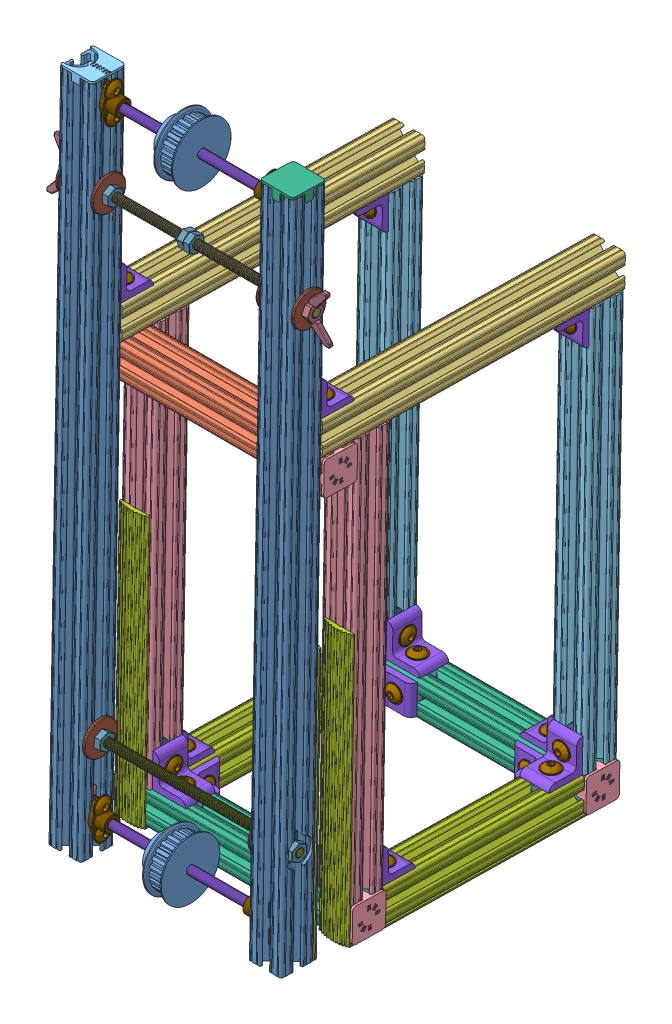
SolidWorks assembly Frame_Assembly_Hardware, configuration Default. Lengths in mm.
Overall size (211.14 529.34 273.97).
180 component instances, 25 part files, 105 mates.
Components (placement in the parent):
- Frame_Extrusions_Assembly-1: Frame_Extrusions_Assembly [Default] at (-237.7441 -252.6867 -297.1575) size (178.82 515.56 261.7)
  - 20in-1: 20in [Default] at (159.5058 -13.8785 410.58) x (1 0 0) z (0 -0.999848 0.017452) size (25.91 25.4 508)
  - 20in-2: 20in [Default] at (311.9058 -13.8785 410.58) x (-1 0 0) z (0 -0.999848 0.017452) size (25.91 25.4 508)
  - 7in_Drilled-1: 7in_Drilled [Default] at (121.4058 325.3515 379.2549) x (0 0.017452 0.999848) z (-1 0 0) size (25.4 25.4 177.8)
  - 9.0625in-1: 9.0625in [Default] at (159.5058 351.4126 416.9058) x (1 0 0) z (0 0.017452 0.999848) size (25.4 25.4 230.19)
  - 9.0625in-2: 9.0625in [Default] at (311.9058 351.4126 416.9058) x (1 0 0) z (0 0.017452 0.999848) size (25.4 25.4 230.19)
  - 12in_Drilled-2: 12in_Drilled [Default] at (159.5058 7.4289 357.8126) x (-1 0 0) z (0 -0.999848 0.017452) size (25.4 25.4 304.8)
  - 12in_Drilled-3: 12in_Drilled [Default] at (311.9058 7.4289 357.8126) x (-1 0 0) z (0 -0.999848 0.017452) size (25.4 25.4 304.8)
  - 12in-1: 12in [Default] at (159.5058 4.3258 180.0397) x (1 0 0) z (0 -0.999848 0.017452) size (25.4 25.4 304.8)
  - 12in-2: 12in [Default] at (311.9058 4.3258 180.0397) x (1 0 0) z (0 -0.999848 0.017452) size (25.4 25.4 304.8)
  - 7in-1: 7in [Default] at (350.0058 20.1269 357.591) x (0 -0.017452 -0.999848) z (1 0 0) size (25.4 25.4 177.8)
  - 7in-2: 7in [Default] at (350.0058 17.0239 179.8181) x (0 -0.017452 -0.999848) z (1 0 0) size (25.4 25.4 177.8)
  - 6in-1: 6in [Default] at (159.5058 20.3486 370.289) x (1 0 0) z (0 0.017452 0.999848) size (25.4 25.4 152.4)
  - 6in-2: 6in [Default] at (311.9058 20.3486 370.289) x (1 0 0) z (0 0.017452 0.999848) size (25.4 25.4 152.4)
- Corner_Brackets_Assembly-1: Corner_Brackets_Assembly [Default] at (64.4635 -222.9732 -111.8459) x (1 0 0) z (0 0.017452 0.999848) size (22.23 33.74 33.74)
  - 2_Hole_Corner_Bracket-1: 2_Hole_Corner_Bracket [Default] at (9.6983 0.1081 6.9858) size (22.23 25.4 25.4)
  - 1_4-20x.5_Flange-1: 1_4-20x.5_Flange [Default] at (9.6983 4.8706 19.6858) x (0 -1 0) z (-0.5 0 0.866025) size (16.15 13.21 13.21)
  - 1_4-20T_Nut-1: 1_4-20T_Nut [Default] at (9.6983 -5.8736 19.6858) x (0 0 1) z (0 -1 0) size (25.4 11.25 3.2)
  - 1_4-20x.5_Flange-2: 1_4-20x.5_Flange [Default] at (9.6983 12.8081 11.7483) x (0 0 -1) z (1 0 0) size (16.15 13.21 13.21)
  - 1_4-20T_Nut-2: 1_4-20T_Nut [Default] at (9.6983 12.8081 1.0041) x (0 1 0) z (0 0 -1) size (25.4 11.25 3.2)
- Corner_Brackets_Assembly-2: Corner_Brackets_Assembly [Default] at (-87.9365 -222.9732 -111.8459) x (1 0 0) z (0 0.017452 0.999848) size (22.23 33.74 33.74)
  - 2_Hole_Corner_Bracket-1: 2_Hole_Corner_Bracket [Default] at (9.6983 0.1081 6.9858) size (22.23 25.4 25.4)
  - 1_4-20x.5_Flange-1: 1_4-20x.5_Flange [Default] at (9.6983 4.8706 19.6858) x (0 -1 0) z (-0.5 0 0.866025) size (16.15 13.21 13.21)
  - 1_4-20T_Nut-1: 1_4-20T_Nut [Default] at (9.6983 -5.8736 19.6858) x (0 0 1) z (0 -1 0) size (25.4 11.25 3.2)
  - 1_4-20x.5_Flange-2: 1_4-20x.5_Flange [Default] at (9.6983 12.8081 11.7483) x (0 0 -1) z (1 0 0) size (16.15 13.21 13.21)
  - 1_4-20T_Nut-2: 1_4-20T_Nut [Default] at (9.6983 12.8081 1.0041) x (0 1 0) z (0 0 -1) size (25.4 11.25 3.2)
- Corner_Brackets_Assembly-3: Corner_Brackets_Assembly [Default] at (83.8601 -220.0696 54.5004) x (-1 0 0) z (0 -0.017452 -0.999848) size (22.23 33.74 33.74)
  - 2_Hole_Corner_Bracket-1: 2_Hole_Corner_Bracket [Default] at (9.6983 0.1081 6.9858) size (22.23 25.4 25.4)
  - 1_4-20x.5_Flange-1: 1_4-20x.5_Flange [Default] at (9.6983 4.8706 19.6858) x (0 -1 0) z (-0.5 0 0.866025) size (16.15 13.21 13.21)
  - 1_4-20T_Nut-1: 1_4-20T_Nut [Default] at (9.6983 -5.8736 19.6858) x (0 0 1) z (0 -1 0) size (25.4 11.25 3.2)
  - 1_4-20x.5_Flange-2: 1_4-20x.5_Flange [Default] at (9.6983 12.8081 11.7483) x (0 0 -1) z (1 0 0) size (16.15 13.21 13.21)
  - 1_4-20T_Nut-2: 1_4-20T_Nut [Default] at (9.6983 12.8081 1.0041) x (0 1 0) z (0 0 -1) size (25.4 11.25 3.2)
- Corner_Brackets_Assembly-4: Corner_Brackets_Assembly [Default] at (-68.5399 -220.0696 54.5004) x (-1 0 0) z (0 -0.017452 -0.999848) size (22.23 33.74 33.74)
  - 2_Hole_Corner_Bracket-1: 2_Hole_Corner_Bracket [Default] at (9.6983 0.1081 6.9858) size (22.23 25.4 25.4)
  - 1_4-20x.5_Flange-1: 1_4-20x.5_Flange [Default] at (9.6983 4.8706 19.6858) x (0 -1 0) z (-0.5 0 0.866025) size (16.15 13.21 13.21)
  - 1_4-20T_Nut-1: 1_4-20T_Nut [Default] at (9.6983 -5.8736 19.6858) x (0 0 1) z (0 -1 0) size (25.4 11.25 3.2)
  - 1_4-20x.5_Flange-2: 1_4-20x.5_Flange [Default] at (9.6983 12.8081 11.7483) x (0 0 -1) z (1 0 0) size (16.15 13.21 13.21)
  - 1_4-20T_Nut-2: 1_4-20T_Nut [Default] at (9.6983 12.8081 1.0041) x (0 1 0) z (0 0 -1) size (25.4 11.25 3.2)
- Corner_Brackets_Assembly-7: Corner_Brackets_Assembly [Default] at (-87.9365 88.9933 -110.4126) x (1 0 0) z (0 -0.999848 0.017452) size (22.23 33.74 33.74)
  - 2_Hole_Corner_Bracket-1: 2_Hole_Corner_Bracket [Default] at (9.6983 0.1081 6.9858) size (22.23 25.4 25.4)
  - 1_4-20x.5_Flange-1: 1_4-20x.5_Flange [Default] at (9.6983 4.8706 19.6858) x (0 -1 0) z (-0.5 0 0.866025) size (16.15 13.21 13.21)
  - 1_4-20T_Nut-1: 1_4-20T_Nut [Default] at (9.6983 -5.8736 19.6858) x (0 0 1) z (0 -1 0) size (25.4 11.25 3.2)
  - 1_4-20x.5_Flange-2: 1_4-20x.5_Flange [Default] at (9.6983 12.8081 11.7483) x (0 0 -1) z (1 0 0) size (16.15 13.21 13.21)
  - 1_4-20T_Nut-2: 1_4-20T_Nut [Default] at (9.6983 12.8081 1.0041) x (0 1 0) z (0 0 -1) size (25.4 11.25 3.2)
- Corner_Brackets_Assembly-8: Corner_Brackets_Assembly [Default] at (64.4635 88.9933 -110.4126) x (1 0 0) z (0 -0.999848 0.017452) size (22.23 33.74 33.74)
  - 2_Hole_Corner_Bracket-1: 2_Hole_Corner_Bracket [Default] at (9.6983 0.1081 6.9858) size (22.23 25.4 25.4)
  - 1_4-20x.5_Flange-1: 1_4-20x.5_Flange [Default] at (9.6983 4.8706 19.6858) x (0 -1 0) z (-0.5 0 0.866025) size (16.15 13.21 13.21)
  - 1_4-20T_Nut-1: 1_4-20T_Nut [Default] at (9.6983 -5.8736 19.6858) x (0 0 1) z (0 -1 0) size (25.4 11.25 3.2)
  - 1_4-20x.5_Flange-2: 1_4-20x.5_Flange [Default] at (9.6983 12.8081 11.7483) x (0 0 -1) z (1 0 0) size (16.15 13.21 13.21)
  - 1_4-20T_Nut-2: 1_4-20T_Nut [Default] at (9.6983 12.8081 1.0041) x (0 1 0) z (0 0 -1) size (25.4 11.25 3.2)
- Corner_Brackets_Assembly-9: Corner_Brackets_Assembly [Default] at (-72.5241 -219.8006 69.9105) x (0 -0.017452 -0.999848) z (1 0 0) size (22.23 33.74 33.74)
  - 2_Hole_Corner_Bracket-1: 2_Hole_Corner_Bracket [Default] at (9.6983 0.1081 6.9858) size (22.23 25.4 25.4)
  - 1_4-20x.5_Flange-1: 1_4-20x.5_Flange [Default] at (9.6983 4.8706 19.6858) x (0 -1 0) z (-0.5 0 0.866025) size (16.15 13.21 13.21)
  - 1_4-20T_Nut-1: 1_4-20T_Nut [Default] at (9.6983 -5.8736 19.6858) x (0 0 1) z (0 -1 0) size (25.4 11.25 3.2)
  - 1_4-20x.5_Flange-2: 1_4-20x.5_Flange [Default] at (9.6983 12.8081 11.7483) x (0 0 -1) z (1 0 0) size (16.15 13.21 13.21)
  - 1_4-20T_Nut-2: 1_4-20T_Nut [Default] at (9.6983 12.8081 1.0041) x (0 1 0) z (0 0 -1) size (25.4 11.25 3.2)
- Corner_Brackets_Assembly-10: Corner_Brackets_Assembly [Default] at (-72.5241 -222.9036 -107.8624) x (0 -0.017452 -0.999848) z (1 0 0) size (22.23 33.74 33.74)
  - 2_Hole_Corner_Bracket-1: 2_Hole_Corner_Bracket [Default] at (9.6983 0.1081 6.9858) size (22.23 25.4 25.4)
  - 1_4-20x.5_Flange-1: 1_4-20x.5_Flange [Default] at (9.6983 4.8706 19.6858) x (0 -1 0) z (-0.5 0 0.866025) size (16.15 13.21 13.21)
  - 1_4-20T_Nut-1: 1_4-20T_Nut [Default] at (9.6983 -5.8736 19.6858) x (0 0 1) z (0 -1 0) size (25.4 11.25 3.2)
  - 1_4-20x.5_Flange-2: 1_4-20x.5_Flange [Default] at (9.6983 12.8081 11.7483) x (0 0 -1) z (1 0 0) size (16.15 13.21 13.21)
  - 1_4-20T_Nut-2: 1_4-20T_Nut [Default] at (9.6983 12.8081 1.0041) x (0 1 0) z (0 0 -1) size (25.4 11.25 3.2)
- Corner_Brackets_Assembly-11: Corner_Brackets_Assembly [Default] at (68.4476 -223.2421 -127.256) x (0 0.017452 0.999848) z (-1 0 0) size (22.23 33.74 33.74)
  - 2_Hole_Corner_Bracket-1: 2_Hole_Corner_Bracket [Default] at (9.6983 0.1081 6.9858) size (22.23 25.4 25.4)
  - 1_4-20x.5_Flange-1: 1_4-20x.5_Flange [Default] at (9.6983 4.8706 19.6858) x (0 -1 0) z (-0.5 0 0.866025) size (16.15 13.21 13.21)
  - 1_4-20T_Nut-1: 1_4-20T_Nut [Default] at (9.6983 -5.8736 19.6858) x (0 0 1) z (0 -1 0) size (25.4 11.25 3.2)
  - 1_4-20x.5_Flange-2: 1_4-20x.5_Flange [Default] at (9.6983 12.8081 11.7483) x (0 0 -1) z (1 0 0) size (16.15 13.21 13.21)
  - 1_4-20T_Nut-2: 1_4-20T_Nut [Default] at (9.6983 12.8081 1.0041) x (0 1 0) z (0 0 -1) size (25.4 11.25 3.2)
- Corner_Brackets_Assembly-12: Corner_Brackets_Assembly [Default] at (68.4476 -220.1391 50.5169) x (0 0.017452 0.999848) z (-1 0 0) size (22.23 33.74 33.74)
  - 2_Hole_Corner_Bracket-1: 2_Hole_Corner_Bracket [Default] at (9.6983 0.1081 6.9858) size (22.23 25.4 25.4)
  - 1_4-20x.5_Flange-1: 1_4-20x.5_Flange [Default] at (9.6983 4.8706 19.6858) x (0 -1 0) z (-0.5 0 0.866025) size (16.15 13.21 13.21)
  - 1_4-20T_Nut-1: 1_4-20T_Nut [Default] at (9.6983 -5.8736 19.6858) x (0 0 1) z (0 -1 0) size (25.4 11.25 3.2)
  - 1_4-20x.5_Flange-2: 1_4-20x.5_Flange [Default] at (9.6983 12.8081 11.7483) x (0 0 -1) z (1 0 0) size (16.15 13.21 13.21)
  - 1_4-20T_Nut-2: 1_4-20T_Nut [Default] at (9.6983 12.8081 1.0041) x (0 1 0) z (0 0 -1) size (25.4 11.25 3.2)
- Corner_Brackets_Assembly-13: Corner_Brackets_Assembly [Default] at (-65.6464 -225.8663 -111.7954) x (0 -0.999848 0.017452) z (0 0.017452 0.999848) size (22.23 33.74 33.74)
  - 2_Hole_Corner_Bracket-1: 2_Hole_Corner_Bracket [Default] at (9.6983 0.1081 6.9858) size (22.23 25.4 25.4)
  - 1_4-20x.5_Flange-1: 1_4-20x.5_Flange [Default] at (9.6983 4.8706 19.6858) x (0 -1 0) z (-0.5 0 0.866025) size (16.15 13.21 13.21)
  - 1_4-20T_Nut-1: 1_4-20T_Nut [Default] at (9.6983 -5.8736 19.6858) x (0 0 1) z (0 -1 0) size (25.4 11.25 3.2)
  - 1_4-20x.5_Flange-2: 1_4-20x.5_Flange [Default] at (9.6983 12.8081 11.7483) x (0 0 -1) z (1 0 0) size (16.15 13.21 13.21)
  - 1_4-20T_Nut-2: 1_4-20T_Nut [Default] at (9.6983 12.8081 1.0041) x (0 1 0) z (0 0 -1) size (25.4 11.25 3.2)
- Corner_Brackets_Assembly-15: Corner_Brackets_Assembly [Default] at (61.5699 -245.2599 -111.4569) x (0 0.999848 -0.017452) z (0 0.017452 0.999848) size (22.23 33.74 33.74)
  - 2_Hole_Corner_Bracket-1: 2_Hole_Corner_Bracket [Default] at (9.6983 0.1081 6.9858) size (22.23 25.4 25.4)
  - 1_4-20x.5_Flange-1: 1_4-20x.5_Flange [Default] at (9.6983 4.8706 19.6858) x (0 -1 0) z (-0.5 0 0.866025) size (16.15 13.21 13.21)
  - 1_4-20T_Nut-1: 1_4-20T_Nut [Default] at (9.6983 -5.8736 19.6858) x (0 0 1) z (0 -1 0) size (25.4 11.25 3.2)
  - 1_4-20x.5_Flange-2: 1_4-20x.5_Flange [Default] at (9.6983 12.8081 11.7483) x (0 0 -1) z (1 0 0) size (16.15 13.21 13.21)
  - 1_4-20T_Nut-2: 1_4-20T_Nut [Default] at (9.6983 12.8081 1.0041) x (0 1 0) z (0 0 -1) size (25.4 11.25 3.2)
- Corner_Brackets_Assembly-16: Corner_Brackets_Assembly [Default] at (68.4476 -242.4764 48.0128) x (0 0.999848 -0.017452) z (-1 0 0) size (22.23 33.74 33.74)
  - 2_Hole_Corner_Bracket-1: 2_Hole_Corner_Bracket [Default] at (9.6983 0.1081 6.9858) size (22.23 25.4 25.4)
  - 1_4-20x.5_Flange-1: 1_4-20x.5_Flange [Default] at (9.6983 4.8706 19.6858) x (0 -1 0) z (-0.5 0 0.866025) size (16.15 13.21 13.21)
  - 1_4-20T_Nut-1: 1_4-20T_Nut [Default] at (9.6983 -5.8736 19.6858) x (0 0 1) z (0 -1 0) size (25.4 11.25 3.2)
  - 1_4-20x.5_Flange-2: 1_4-20x.5_Flange [Default] at (9.6983 12.8081 11.7483) x (0 0 -1) z (1 0 0) size (16.15 13.21 13.21)
  - 1_4-20T_Nut-2: 1_4-20T_Nut [Default] at (9.6983 12.8081 1.0041) x (0 1 0) z (0 0 -1) size (25.4 11.25 3.2)
- Corner_Brackets_Assembly-18: Corner_Brackets_Assembly [Default] at (-72.5241 -223.0827 47.6743) x (0 -0.999848 0.017452) z (1 0 0) size (22.23 33.74 33.74)
  - 2_Hole_Corner_Bracket-1: 2_Hole_Corner_Bracket [Default] at (9.6983 0.1081 6.9858) size (22.23 25.4 25.4)
  - 1_4-20x.5_Flange-1: 1_4-20x.5_Flange [Default] at (9.6983 4.8706 19.6858) x (0 -1 0) z (-0.5 0 0.866025) size (16.15 13.21 13.21)
  - 1_4-20T_Nut-1: 1_4-20T_Nut [Default] at (9.6983 -5.8736 19.6858) x (0 0 1) z (0 -1 0) size (25.4 11.25 3.2)
  - 1_4-20x.5_Flange-2: 1_4-20x.5_Flange [Default] at (9.6983 12.8081 11.7483) x (0 0 -1) z (1 0 0) size (16.15 13.21 13.21)
  - 1_4-20T_Nut-2: 1_4-20T_Nut [Default] at (9.6983 12.8081 1.0041) x (0 1 0) z (0 0 -1) size (25.4 11.25 3.2)
- Corner_Brackets_Assembly-19: Corner_Brackets_Assembly [Default] at (83.8601 110.9944 101.1172) x (-1 0 0) z (0 -0.017452 -0.999848) size (22.23 33.74 33.74)
  - 2_Hole_Corner_Bracket-1: 2_Hole_Corner_Bracket [Default] at (9.6983 0.1081 6.9858) size (22.23 25.4 25.4)
  - 1_4-20x.5_Flange-1: 1_4-20x.5_Flange [Default] at (9.6983 4.8706 19.6858) x (0 -1 0) z (-0.5 0 0.866025) size (16.15 13.21 13.21)
  - 1_4-20T_Nut-1: 1_4-20T_Nut [Default] at (9.6983 -5.8736 19.6858) x (0 0 1) z (0 -1 0) size (25.4 11.25 3.2)
  - 1_4-20x.5_Flange-2: 1_4-20x.5_Flange [Default] at (9.6983 12.8081 11.7483) x (0 0 -1) z (1 0 0) size (16.15 13.21 13.21)
  - 1_4-20T_Nut-2: 1_4-20T_Nut [Default] at (9.6983 12.8081 1.0041) x (0 1 0) z (0 0 -1) size (25.4 11.25 3.2)
- Corner_Brackets_Assembly-20: Corner_Brackets_Assembly [Default] at (-68.5399 110.9944 101.1172) x (-1 0 0) z (0 -0.017452 -0.999848) size (22.23 33.74 33.74)
  - 2_Hole_Corner_Bracket-1: 2_Hole_Corner_Bracket [Default] at (9.6983 0.1081 6.9858) size (22.23 25.4 25.4)
  - 1_4-20x.5_Flange-1: 1_4-20x.5_Flange [Default] at (9.6983 4.8706 19.6858) x (0 -1 0) z (-0.5 0 0.866025) size (16.15 13.21 13.21)
  - 1_4-20T_Nut-1: 1_4-20T_Nut [Default] at (9.6983 -5.8736 19.6858) x (0 0 1) z (0 -1 0) size (25.4 11.25 3.2)
  - 1_4-20x.5_Flange-2: 1_4-20x.5_Flange [Default] at (9.6983 12.8081 11.7483) x (0 0 -1) z (1 0 0) size (16.15 13.21 13.21)
  - 1_4-20T_Nut-2: 1_4-20T_Nut [Default] at (9.6983 12.8081 1.0041) x (0 1 0) z (0 0 -1) size (25.4 11.25 3.2)
- Top_Brace_Assembly-1: Top_Brace_Assembly [Default] at (73.3092 178.2963 87.425) size (211.14 38.15 32.33)
  - 1in_0.25_FenderWasher-1: 1in_0.25_FenderWasher [Default] at (13.5526 12.2689 18.0183) size (1.59 25.4 25.4)
  - 1in_0.25_FenderWasher-2: 1in_0.25_FenderWasher [Default] at (-164.2474 12.2689 18.0183) x (-1 0 0) z (0 -0.17346 -0.984841) size (1.59 25.4 25.4)
  - Top_Brace_Rod-1: Top_Brace_Rod [Default] at (-176.9474 12.2814 17.9931) size (193.16 7.33 6.54)
  - 7_16-1_4-20_WingNut-1: 7_16-1_4-20_WingNut [Default] at (-170.5974 12.2689 18.0183) x (1 0 0) z (0 -0.985852 0.167617) size (15.26 12.83 36.51)
  - 7_16-1_4-20_WingNut-2: 7_16-1_4-20_WingNut [Default] at (19.9026 12.2689 18.0183) x (-1 0 0) z (0 -0.99807 -0.062096) size (15.26 12.83 36.51)
  - 7_16-1_4-20_Nut-1: 7_16-1_4-20_Nut [Default] at (-80.4274 12.2689 18.0183) x (1 0 0) z (0 -0.962859 0.270005) size (4.94 12.83 11.11)
  - 7_16-1_4-20_Nut-2: 7_16-1_4-20_Nut [Default] at (-75.6649 12.2689 18.0183) x (1 0 0) z (0 -0.117902 0.993025) size (4.94 12.83 11.11)
  - 1in_0.25_FenderWasher-3: 1in_0.25_FenderWasher [Default] at (-138.8474 12.2689 18.0183) x (1 0 0) z (0 -0.328292 0.944576) size (1.59 25.4 25.4)
  - 1in_0.25_FenderWasher-4: 1in_0.25_FenderWasher [Default] at (-11.8474 12.2689 18.0183) x (-1 0 0) z (0 -0.17346 -0.984841) size (1.59 25.4 25.4)
  - 7_16-1_4-20_Nut-3: 7_16-1_4-20_Nut [Default] at (-137.2599 12.2689 18.0183) size (4.94 12.83 11.11)
  - 7_16-1_4-20_Nut-4: 7_16-1_4-20_Nut [Default] at (-18.1974 12.2689 18.0183) x (1 0 0) z (0 -0.311077 0.950385) size (4.94 12.83 11.11)
- Bottom_Brace_Slide_Washer-1: Bottom_Brace_Slide_Washer [Default] at (78.6576 -164.9806 111.6494) x (1 0 0) z (0 0.017452 0.999848) size (1.78 19.05 12.7)
- Bottom_Brace_Slide_Washer-2: Bottom_Brace_Slide_Washer [Default] at (-84.512 -164.9806 111.6494) x (1 0 0) z (0 0.017452 0.999848) size (1.78 19.05 12.7)
- Bottom_Brace_Assembly-1: Bottom_Brace_Assembly [Default] at (-71.3975 -254.0686 -29.1718) size (180.38 29.74 29.74)
  - Bottom_Brace_Rod-1: Bottom_Brace_Rod [Default] at (-25.8907 88.9737 140.9504) size (180.38 7.33 6.54)
  - 7_16-1_4-20_Nut-1: 7_16-1_4-20_Nut [Default] at (153.4968 89.0879 140.8212) size (4.94 12.83 11.11)
  - 7_16-1_4-20_Nut-2: 7_16-1_4-20_Nut [Default] at (-19.5407 89.0879 140.8212) x (1 0 0) z (0 -0.663965 0.747764) size (4.94 12.83 11.11)
  - 1in_0.25_FenderWasher-1: 1in_0.25_FenderWasher [Default] at (5.8593 89.0879 140.8212) x (1 0 0) z (0 -0.188999 0.981977) size (1.59 25.4 25.4)
  - 1in_0.25_FenderWasher-2: 1in_0.25_FenderWasher [Default] at (132.8593 89.0879 140.8212) x (-1 0 0) z (0 0.002383 -0.999997) size (1.59 25.4 25.4)
  - 7_16-1_4-20_Nut-3: 7_16-1_4-20_Nut [Default] at (126.5093 89.0879 140.8212) x (1 0 0) z (0 -0.998838 0.048199) size (4.94 12.83 11.11)
  - 7_16-1_4-20_Nut-4: 7_16-1_4-20_Nut [Default] at (7.4468 89.0879 140.8212) x (1 0 0) z (0 0.082166 0.996619) size (4.94 12.83 11.11)
- Pulley_Assembly-1: Pulley_Assembly [Default] at (-69.0635 -272.8603 -5.2979) x (0.999962 0.008726 -0.000076) z (0.000076 0.000001 1) size (147.14 50.64 50.44)
  - Pulley_Shaft-1: Pulley_Shaft [Default] at (7.1831 56.3247 118.0204) x (0.999962 -0.008726 0.000076) z (-0.000076 0 1) size (120.65 6.35 6.35)
  - Babbit_Bearing-1: Babbit_Bearing [2943N3] at (131.7971 55.2372 118.0299) x (0.008727 0.999924 -0.008726) z (0.999962 -0.008726 0.000076) size (25.09 15.08 11.11)
  - Babbit_Bearing-2: Babbit_Bearing [2943N3] at (3.2145 56.3593 118.0201) x (-0.008724 -0.999867 -0.013791) z (-0.999962 0.008726 -0.000076) size (25.09 15.08 11.11)
  - 1_4-20x.5_Flange-1: 1_4-20x.5_Flange [Default] at (127.9047 64.0025 117.9534) x (0.999962 -0.008726 0.000076) z (-0.008441 -0.964941 0.262332) size (16.15 13.21 13.21)
  - 1_4-20x.5_Flange-2: 1_4-20x.5_Flange [Default] at (127.7523 46.5413 118.1057) x (0.999962 -0.008726 0.000076) z (-0.008441 -0.964941 0.262332) size (16.15 13.21 13.21)
  - 1_4-20x.5_Flange-3: 1_4-20x.5_Flange [Default] at (7.2593 65.0548 118.1408) x (-0.999962 0.008726 -0.000076) z (-0.008401 -0.964941 -0.262333) size (16.15 13.21 13.21)
  - Timing_Pulley-1: Timing_Pulley [1277N51] at (62.9848 55.8377 118.0246) x (0.008645 0.989349 -0.145305) z (-0.999962 0.008726 -0.000076) size (44.45 44.45 23.01)
  - 1_4-20T_Nut_Truncated-1: 1_4-20T_Nut_Truncated [Default] at (138.6485 63.9087 117.9542) x (0.008726 0.99981 -0.017452) z (0.999962 -0.008726 0.000076) size (14.15 11.25 3.2)
  - 1_4-20T_Nut_Truncated-2: 1_4-20T_Nut_Truncated [Default] at (138.4961 46.4475 118.1066) x (0.008726 0.99981 -0.017452) z (0.999962 -0.008726 0.000076) size (14.15 11.25 3.2)
  - 1_4-20x.5_Flange-5: 1_4-20x.5_Flange [Default] at (7.1069 47.5946 117.9) x (-0.999962 0.008726 -0.000076) z (-0.008401 -0.964941 -0.262333) size (16.15 13.21 13.21)
  - 1_4-20T_Nut_Truncated-3: 1_4-20T_Nut_Truncated [Default] at (-3.4845 65.1485 118.14) x (0.008724 0.99981 0.017453) z (-0.999962 0.008726 -0.000076) size (14.15 11.25 3.2)
  - 1_4-20T_Nut_Truncated-4: 1_4-20T_Nut_Truncated [Default] at (-3.6369 47.6884 117.8991) x (0.008724 0.99981 0.017453) z (-0.999962 0.008726 -0.000076) size (14.15 11.25 3.2)
- Pulley_Assembly-2: Pulley_Assembly [Default] at (-69.0635 194.5622 -13.8406) x (0.999962 0.008726 -0.000076) z (0.000076 0.000001 1) size (147.14 50.64 50.44)
  - Pulley_Shaft-1: Pulley_Shaft [Default] at (7.1831 56.3247 118.0204) x (0.999962 -0.008726 0.000076) z (-0.000076 0 1) size (120.65 6.35 6.35)
  - Babbit_Bearing-1: Babbit_Bearing [2943N3] at (131.7971 55.2372 118.0299) x (0.008727 0.999924 -0.008726) z (0.999962 -0.008726 0.000076) size (25.09 15.08 11.11)
  - Babbit_Bearing-2: Babbit_Bearing [2943N3] at (3.2145 56.3593 118.0201) x (-0.008724 -0.999867 -0.013791) z (-0.999962 0.008726 -0.000076) size (25.09 15.08 11.11)
  - 1_4-20x.5_Flange-1: 1_4-20x.5_Flange [Default] at (127.9047 64.0025 117.9534) x (0.999962 -0.008726 0.000076) z (-0.008441 -0.964941 0.262332) size (16.15 13.21 13.21)
  - 1_4-20x.5_Flange-2: 1_4-20x.5_Flange [Default] at (127.7523 46.5413 118.1057) x (0.999962 -0.008726 0.000076) z (-0.008441 -0.964941 0.262332) size (16.15 13.21 13.21)
  - 1_4-20x.5_Flange-3: 1_4-20x.5_Flange [Default] at (7.2593 65.0548 118.1408) x (-0.999962 0.008726 -0.000076) z (-0.008401 -0.964941 -0.262333) size (16.15 13.21 13.21)
  - Timing_Pulley-1: Timing_Pulley [1277N51] at (62.9848 55.8377 118.0246) x (0.008645 0.989349 -0.145305) z (-0.999962 0.008726 -0.000076) size (44.45 44.45 23.01)
  - 1_4-20T_Nut_Truncated-1: 1_4-20T_Nut_Truncated [Default] at (138.6485 63.9087 117.9542) x (0.008726 0.99981 -0.017452) z (0.999962 -0.008726 0.000076) size (14.15 11.25 3.2)
  - 1_4-20T_Nut_Truncated-2: 1_4-20T_Nut_Truncated [Default] at (138.4961 46.4475 118.1066) x (0.008726 0.99981 -0.017452) z (0.999962 -0.008726 0.000076) size (14.15 11.25 3.2)
  - 1_4-20x.5_Flange-5: 1_4-20x.5_Flange [Default] at (7.1069 47.5946 117.9) x (-0.999962 0.008726 -0.000076) z (-0.008401 -0.964941 -0.262333) size (16.15 13.21 13.21)
  - 1_4-20T_Nut_Truncated-3: 1_4-20T_Nut_Truncated [Default] at (-3.4845 65.1485 118.14) x (0.008724 0.99981 0.017453) z (-0.999962 0.008726 -0.000076) size (14.15 11.25 3.2)
  - 1_4-20T_Nut_Truncated-4: 1_4-20T_Nut_Truncated [Default] at (-3.6369 47.6884 117.8991) x (0.008724 0.99981 0.017453) z (-0.999962 0.008726 -0.000076) size (14.15 11.25 3.2)
- Through_Bolt-1: Through_Bolt [Default] at (97.6342 81.6926 62.1337) x (1 0 0) z (0 0.017452 0.999848) size (13.08 26.15 64.27)
  - Shoulder_Bolt-1: Shoulder_Bolt [90128A254] at (-23.4724 -9.1964 43.6156) size (9.53 9.53 64.27)
  - 1_4-20T_Nut-1: 1_4-20T_Nut [Default] at (-23.4724 -9.1964 39.2468) x (-0.073084 -0.997326 0) z (0 0 1) size (25.4 11.25 3.2)
- 1in_0.25_FenderWasher-1: 1in_0.25_FenderWasher [Default] at (74.1618 72.6216 69.3962) x (0 -0.017452 -0.999848) z (1 -0.000076 0.000001) size (1.59 25.4 25.4)
- 1in_0.25_FenderWasher-2: 1in_0.25_FenderWasher [Default] at (-78.2382 72.6216 69.3962) x (0 -0.017452 -0.999848) z (1 -0.000076 0.000001) size (1.59 25.4 25.4)
- Through_Bolt-2: Through_Bolt [Default] at (-101.7107 63.3027 62.4547) x (-1 0 0) z (0 0.017452 0.999848) size (13.08 26.15 64.27)
  - Shoulder_Bolt-1: Shoulder_Bolt [90128A254] at (-23.4724 -9.1964 43.6156) size (9.53 9.53 64.27)
  - 1_4-20T_Nut-1: 1_4-20T_Nut [Default] at (-23.4724 -9.1964 39.2468) x (-0.073084 -0.997326 0) z (0 0 1) size (25.4 11.25 3.2)
- 8020_Encaps-1: 8020_Encaps [Default] at (88.4493 72.6648 82.0974) x (0 -0.017452 -0.999848) z (-1 0 0) size (25.4 25.4 14.29)
- 8020_Encaps-2: 8020_Encaps [Default] at (88.4493 -232.5598 60.4335) x (0 -0.017452 -0.999848) z (-1 0 0) size (25.4 25.4 14.29)
- 8020_Encaps-3: 8020_Encaps [Default] at (88.4493 -235.6628 -117.3394) x (0 -0.017452 -0.999848) z (-1 0 0) size (25.4 25.4 14.29)
- 8020_Encaps-4: 8020_Encaps [Default] at (-92.5257 72.6648 82.0974) x (0 0 -1) z (1 0 0) size (25.4 25.4 14.29)
- 8020_Encaps-5: 8020_Encaps [Default] at (-92.5257 -232.5598 60.4335) x (0 0 -1) z (1 0 0) size (25.4 25.4 14.29)
- 8020_Encaps-6: 8020_Encaps [Default] at (-92.5257 -235.6628 -117.3394) x (0 0 -1) z (1 0 0) size (25.4 25.4 14.29)
- 8020_Encaps_Limit_Side-1: 8020_Encaps_Limit_Side [Default] at (-78.2382 268.3408 104.0857) x (-1 0 0) z (0 -0.999848 0.017452) size (25.22 25.4 14.29)
- 8020_Encaps_Flat-1: 8020_Encaps_Flat [Default] at (74.1618 268.3408 104.0857) x (-0.999962 -0.000152 -0.008726) z (0 -0.999848 0.017452) size (25.4 25.4 14.29)
- Tread_8in-1: Tread_8in [Default] at (75.7493 -244.944 -282.3026) x (-1 0 0) z (0 0.017452 0.999848) size (22.23 10.11 203.2)
- Tread_8in-2: Tread_8in [Default] at (-79.8257 -244.944 -282.3026) x (-1 0 0) z (0 0.017452 0.999848) size (22.23 10.11 203.2)
- Tread_8in-3: Tread_8in [Default] at (-79.8257 -393.6575 109.2392) x (1 0 0) z (0 0.999848 -0.017452) size (22.23 10.11 203.2)
- Tread_8in-4: Tread_8in [Default] at (75.7493 -393.6575 109.2392) x (1 0 0) z (0 0.999848 -0.017452) size (22.23 10.11 203.2)
- Tread_8in-5: Tread_8in [Default] at (75.7493 -397.5229 69.7147) x (-1 0 0) z (0 0.999848 -0.017452) size (22.23 10.11 203.2)
- Tread_8in-6: Tread_8in [Default] at (-79.8257 -397.5229 69.7147) x (-1 0 0) z (0 0.999848 -0.017452) size (22.23 10.11 203.2)
Mates (geometry in assembly coordinates):
- Coincident2: coincident anti-aligned: plane of Frame_Extrusions_Assembly-1/6in-2 through (80.4948 -222.7431 -104.863) normal (0 0.999848 -0.017452); plane of Corner_Brackets_Assembly-1/2_Hole_Corner_Bracket-1 through (85.2743 -222.2998 -79.4669) normal (0 -0.999848 0.017452)
- Coincident3: coincident anti-aligned: plane of Frame_Extrusions_Assembly-1/12in-2 through (80.4948 82.0105 -110.1825) normal (0 0.017452 0.999848); plane of Corner_Brackets_Assembly-1/2_Hole_Corner_Bracket-1 through (85.2743 -222.7431 -104.863) normal (0 -0.017452 -0.999848)
- Coincident4: coincident anti-aligned: plane of Frame_Extrusions_Assembly-1/12in-1 through (-71.9052 82.0105 -110.1825) normal (0 0.017452 0.999848); plane of Corner_Brackets_Assembly-2/2_Hole_Corner_Bracket-1 through (-67.1257 -222.7431 -104.863) normal (0 -0.017452 -0.999848)
- Coincident6: coincident anti-aligned: plane of Frame_Extrusions_Assembly-1/6in-1 through (-71.9052 -222.7431 -104.863) normal (0 0.999848 -0.017452); plane of Corner_Brackets_Assembly-2/2_Hole_Corner_Bracket-1 through (-67.1257 -222.2998 -79.4669) normal (0 -0.999848 0.017452)
- Coincident8: coincident anti-aligned: plane of Frame_Extrusions_Assembly-1/12in_Drilled-3 through (83.7122 84.6702 42.1943) normal (0 -0.017452 -0.999848); plane of Corner_Brackets_Assembly-3/2_Hole_Corner_Bracket-1 through (63.0493 -220.0834 47.5138) normal (0 0.017452 0.999848)
- Coincident9: coincident anti-aligned: plane of Frame_Extrusions_Assembly-1/6in-2 through (80.4948 -222.7431 -104.863) normal (0 0.999848 -0.017452); plane of Corner_Brackets_Assembly-3/2_Hole_Corner_Bracket-1 through (63.0493 -220.5266 22.1176) normal (0 -0.999848 0.017452)
- Coincident11: coincident anti-aligned: plane of Frame_Extrusions_Assembly-1/6in-1 through (-71.9052 -222.7431 -104.863) normal (0 0.999848 -0.017452); plane of Corner_Brackets_Assembly-4/2_Hole_Corner_Bracket-1 through (-89.3507 -220.5266 22.1176) normal (0 -0.999848 0.017452)
- Coincident12: coincident anti-aligned: plane of Frame_Extrusions_Assembly-1/12in_Drilled-2 through (-68.6878 84.6702 42.1943) normal (0 -0.017452 -0.999848); plane of Corner_Brackets_Assembly-4/2_Hole_Corner_Bracket-1 through (-89.3507 -220.0834 47.5138) normal (0 0.017452 0.999848)
- Coincident21: coincident anti-aligned: plane of Frame_Extrusions_Assembly-1/9.0625in-1 through (-84.5713 81.5672 -135.5786) normal (0 -0.999848 0.017452); plane of Corner_Brackets_Assembly-7/2_Hole_Corner_Bracket-1 through (-67.1257 82.0105 -110.1825) normal (0 0.999848 -0.017452)
- Coincident22: coincident anti-aligned: plane of Frame_Extrusions_Assembly-1/12in-1 through (-87.7886 82.0105 -110.1825) normal (0 0.017452 0.999848); plane of Corner_Brackets_Assembly-7/2_Hole_Corner_Bracket-1 through (-67.1257 56.6143 -109.7392) normal (0 -0.017452 -0.999848)
- Coincident26: coincident anti-aligned: plane of Frame_Extrusions_Assembly-1/9.0625in-2 through (83.7122 81.5672 -135.5786) normal (0 -0.999848 0.017452); plane of Corner_Brackets_Assembly-8/2_Hole_Corner_Bracket-1 through (85.2743 82.0105 -110.1825) normal (0 0.999848 -0.017452)
- Coincident27: coincident anti-aligned: plane of Frame_Extrusions_Assembly-1/12in-2 through (80.4948 82.0105 -110.1825) normal (0 0.017452 0.999848); plane of Corner_Brackets_Assembly-8/2_Hole_Corner_Bracket-1 through (85.2743 56.6143 -109.7392) normal (0 -0.017452 -0.999848)
- Coincident32: coincident anti-aligned: plane of Frame_Extrusions_Assembly-1/7in-1 through (-90.9382 -219.695 69.7608) normal (0 0.999848 -0.017452); plane of Corner_Brackets_Assembly-9/2_Hole_Corner_Bracket-1 through (-40.1382 -220.0557 49.101) normal (0 -0.999848 0.017452)
- Coincident33: coincident anti-aligned: plane of Frame_Extrusions_Assembly-1/12in_Drilled-2 through (-65.5382 85.0585 64.4413) normal (1 0 0); plane of Corner_Brackets_Assembly-9/2_Hole_Corner_Bracket-1 through (-65.5382 -220.0557 49.101) normal (-1 0 0)
- Distance2: distance = 1.5875 mm aligned: plane of Corner_Brackets_Assembly-9/2_Hole_Corner_Bracket-1 through (-44.9007 -219.6678 71.3226) normal (0 0.017452 0.999848); plane of Frame_Extrusions_Assembly-1/7in-1 through (-90.9382 -226.006 73.021) normal (0 0.017452 0.999848)
- Distance3: distance = 1.5875 mm aligned: plane of Corner_Brackets_Assembly-4/2_Hole_Corner_Bracket-1 through (-89.3507 -220.4435 26.8794) normal (-1 0 0); plane of Frame_Extrusions_Assembly-1/6in-1 through (-90.9382 -229.1091 -104.7519) normal (-1 0 0)
- Distance5: distance = 1.5875 mm aligned: plane of Corner_Brackets_Assembly-3/2_Hole_Corner_Bracket-1 through (85.2743 -220.4435 26.8794) normal (1 0 0); plane of Frame_Extrusions_Assembly-1/6in-2 through (86.8618 -225.8922 -104.808) normal (1 0 0)
- Distance6: distance = 1.5875 mm aligned: plane of Corner_Brackets_Assembly-1/2_Hole_Corner_Bracket-1 through (85.2743 -222.3829 -84.2287) normal (1 0 0); plane of Frame_Extrusions_Assembly-1/6in-2 through (86.8618 -225.8922 -104.808) normal (1 0 0)
- Distance8: distance = 1.5875 mm aligned: plane of Corner_Brackets_Assembly-8/2_Hole_Corner_Bracket-1 through (85.2743 61.3761 -109.8223) normal (1 0 0); plane of Frame_Extrusions_Assembly-1/9.0625in-2 through (86.8618 87.9331 -135.6898) normal (1 0 0)
- Distance11: distance = 1.5875 mm aligned: plane of Corner_Brackets_Assembly-7/2_Hole_Corner_Bracket-1 through (-89.3507 61.3761 -109.8223) normal (-1 0 0); plane of Frame_Extrusions_Assembly-1/9.0625in-1 through (-90.9382 84.7163 -135.6336) normal (-1 0 0)
- Distance12: distance = 1.5875 mm aligned: plane of Corner_Brackets_Assembly-2/2_Hole_Corner_Bracket-1 through (-89.3507 -222.3829 -84.2287) normal (-1 0 0); plane of Frame_Extrusions_Assembly-1/6in-1 through (-90.9382 -229.1091 -104.7519) normal (-1 0 0)
- Distance13: distance = 1.5875 mm aligned: plane of Corner_Brackets_Assembly-10/2_Hole_Corner_Bracket-1 through (-44.9007 -223.1587 -128.6719) normal (0 -0.017452 -0.999848); plane of Frame_Extrusions_Assembly-1/7in-2 through (-90.9382 -226.3355 -130.2042) normal (0 -0.017452 -0.999848)
- Coincident34: coincident anti-aligned: plane of Frame_Extrusions_Assembly-1/12in-1 through (-65.5382 81.6783 -129.2127) normal (1 0 0); plane of Corner_Brackets_Assembly-10/2_Hole_Corner_Bracket-1 through (-65.5382 -223.1587 -128.6719) normal (-1 0 0)
- Coincident35: coincident anti-aligned: plane of Frame_Extrusions_Assembly-1/7in-2 through (-90.9382 -223.0753 -123.8932) normal (0 0.999848 -0.017452); plane of Corner_Brackets_Assembly-10/2_Hole_Corner_Bracket-1 through (-40.1382 -223.1587 -128.6719) normal (0 -0.999848 0.017452)
- Coincident36: coincident anti-aligned: plane of Frame_Extrusions_Assembly-1/12in-2 through (61.4618 81.6221 -132.4295) normal (-1 0 0); plane of Corner_Brackets_Assembly-11/2_Hole_Corner_Bracket-1 through (61.4618 -222.7708 -106.4503) normal (1 0 0)
- Coincident37: coincident anti-aligned: plane of Frame_Extrusions_Assembly-1/7in-2 through (-90.9382 -223.0753 -123.8932) normal (0 0.999848 -0.017452); plane of Corner_Brackets_Assembly-11/2_Hole_Corner_Bracket-1 through (36.0618 -222.7708 -106.4503) normal (0 -0.999848 0.017452)
- Distance14: distance = 1.5875 mm aligned: plane of Corner_Brackets_Assembly-11/2_Hole_Corner_Bracket-1 through (40.8243 -223.1587 -128.6719) normal (0 -0.017452 -0.999848); plane of Frame_Extrusions_Assembly-1/7in-2 through (-90.9382 -226.3355 -130.2042) normal (0 -0.017452 -0.999848)
- Coincident38: coincident anti-aligned: plane of Frame_Extrusions_Assembly-1/7in-1 through (-90.9382 -219.695 69.7608) normal (0 0.999848 -0.017452); plane of Corner_Brackets_Assembly-12/2_Hole_Corner_Bracket-1 through (36.0618 -219.6678 71.3226) normal (0 -0.999848 0.017452)
- Coincident39: coincident anti-aligned: plane of Frame_Extrusions_Assembly-1/12in_Drilled-3 through (61.4618 85.0024 61.2245) normal (-1 0 0); plane of Corner_Brackets_Assembly-12/2_Hole_Corner_Bracket-1 through (61.4618 -219.6678 71.3226) normal (1 0 0)
- Distance16: distance = 1.5875 mm aligned: plane of Corner_Brackets_Assembly-12/2_Hole_Corner_Bracket-1 through (40.8243 -219.6678 71.3226) normal (0 0.017452 0.999848); plane of Frame_Extrusions_Assembly-1/7in-1 through (-90.9382 -226.006 73.021) normal (0 0.017452 0.999848)
- Coincident40: coincident anti-aligned: plane of Frame_Extrusions_Assembly-1/6in-1 through (-65.5382 -225.8922 -104.808) normal (1 0 0); plane of Corner_Brackets_Assembly-13/2_Hole_Corner_Bracket-1 through (-65.5382 -246.1087 -79.0513) normal (-1 0 0)
- Coincident41: coincident anti-aligned: plane of Frame_Extrusions_Assembly-1/7in-2 through (-90.9382 -229.1091 -104.7519) normal (0 0.017452 0.999848); plane of Corner_Brackets_Assembly-13/2_Hole_Corner_Bracket-1 through (-65.5382 -246.552 -104.4474) normal (0 -0.017452 -0.999848)
- Distance17: distance = 1.5875 mm aligned: plane of Corner_Brackets_Assembly-13/2_Hole_Corner_Bracket-1 through (-65.5382 -223.9702 -84.201) normal (0 0.999848 -0.017452); plane of Frame_Extrusions_Assembly-1/7in-2 through (-90.9382 -222.7981 -108.0121) normal (0 0.999848 -0.017452)
- Coincident42: coincident anti-aligned: plane of Frame_Extrusions_Assembly-1/7in-2 through (-90.9382 -229.1091 -104.7519) normal (0 0.017452 0.999848); plane of Corner_Brackets_Assembly-15/2_Hole_Corner_Bracket-1 through (61.4618 -224.3304 -104.8353) normal (0 -0.017452 -0.999848)
- Coincident43: coincident anti-aligned: plane of Frame_Extrusions_Assembly-1/6in-2 through (61.4618 -229.1091 -104.7519) normal (-1 0 0); plane of Corner_Brackets_Assembly-15/2_Hole_Corner_Bracket-1 through (61.4618 -223.8871 -79.4392) normal (1 0 0)
- Distance18: distance = 1.5875 mm aligned: plane of Corner_Brackets_Assembly-15/2_Hole_Corner_Bracket-1 through (61.4618 -223.9702 -84.201) normal (0 0.999848 -0.017452); plane of Frame_Extrusions_Assembly-1/7in-2 through (-90.9382 -222.7981 -108.0121) normal (0 0.999848 -0.017452)
- Coincident44: coincident anti-aligned: plane of Frame_Extrusions_Assembly-1/7in-1 through (-90.9382 -223.2325 47.5687) normal (0 -0.017452 -0.999848); plane of Corner_Brackets_Assembly-16/2_Hole_Corner_Bracket-1 through (36.0618 -221.6706 47.5415) normal (0 0.017452 0.999848)
- Coincident45: coincident anti-aligned: plane of Frame_Extrusions_Assembly-1/6in-2 through (61.4618 -229.1091 -104.7519) normal (-1 0 0); plane of Corner_Brackets_Assembly-16/2_Hole_Corner_Bracket-1 through (61.4618 -221.6706 47.5415) normal (1 0 0)
- Distance19: distance = 1.5875 mm aligned: plane of Corner_Brackets_Assembly-16/2_Hole_Corner_Bracket-1 through (40.8243 -221.6706 47.5415) normal (0 0.999848 -0.017452); plane of Frame_Extrusions_Assembly-1/6in-2 through (64.6114 -222.7431 -104.863) normal (0 0.999848 -0.017452)
- Coincident46: coincident anti-aligned: plane of Frame_Extrusions_Assembly-1/6in-1 through (-65.5382 -225.8922 -104.808) normal (1 0 0); plane of Corner_Brackets_Assembly-18/2_Hole_Corner_Bracket-1 through (-65.5382 -243.8922 47.9294) normal (-1 0 0)
- Coincident47: coincident anti-aligned: plane of Frame_Extrusions_Assembly-1/7in-1 through (-90.9382 -223.2325 47.5687) normal (0 -0.017452 -0.999848); plane of Corner_Brackets_Assembly-18/2_Hole_Corner_Bracket-1 through (-40.1382 -243.8922 47.9294) normal (0 0.017452 0.999848)
- Distance20: distance = 1.5875 mm aligned: plane of Corner_Brackets_Assembly-18/2_Hole_Corner_Bracket-1 through (-44.9007 -221.6706 47.5415) normal (0 0.999848 -0.017452); plane of Frame_Extrusions_Assembly-1/6in-1 through (-71.9052 -222.7431 -104.863) normal (0 0.999848 -0.017452)
- Coincident48: coincident anti-aligned: plane of Frame_Extrusions_Assembly-1/9.0625in-2 through (80.4948 106.9633 -136.0219) normal (0 0.999848 -0.017452); plane of Corner_Brackets_Assembly-19/2_Hole_Corner_Bracket-1 through (63.0493 110.5373 68.7344) normal (0 -0.999848 0.017452)
- Coincident49: coincident anti-aligned: plane of Frame_Extrusions_Assembly-1/20in-2 through (83.7122 266.5319 91.4153) normal (0 -0.017452 -0.999848); plane of Corner_Brackets_Assembly-19/2_Hole_Corner_Bracket-1 through (63.0493 110.9806 94.1305) normal (0 0.017452 0.999848)
- Coincident51: coincident anti-aligned: plane of Frame_Extrusions_Assembly-1/9.0625in-1 through (-87.7886 106.9633 -136.0219) normal (0 0.999848 -0.017452); plane of Corner_Brackets_Assembly-20/2_Hole_Corner_Bracket-1 through (-89.3507 110.5373 68.7344) normal (0 -0.999848 0.017452)
- Coincident52: coincident anti-aligned: plane of Frame_Extrusions_Assembly-1/20in-1 through (-84.5713 266.5319 91.4153) normal (0 -0.017452 -0.999848); plane of Corner_Brackets_Assembly-20/2_Hole_Corner_Bracket-1 through (-89.3507 110.9806 94.1305) normal (0 0.017452 0.999848)
- Distance23: distance = 1.5875 mm aligned: plane of Corner_Brackets_Assembly-19/2_Hole_Corner_Bracket-1 through (85.2743 110.6205 73.4962) normal (1 0 0); plane of Frame_Extrusions_Assembly-1/9.0625in-2 through (86.8618 103.8142 -135.967) normal (1 0 0)
- Coincident53: coincident anti-aligned: plane of Frame_Extrusions_Assembly-1/20in-2 through (61.4618 266.5869 94.5645) normal (-1 0 0); plane of Top_Brace_Assembly-1/1in_0.25_FenderWasher-4 through (61.4618 190.5652 105.4433) normal (1 0 0)
- Concentric1: concentric anti-aligned: cylinder of Frame_Extrusions_Assembly-1/20in-1 through (-101.7145 190.5652 105.4433) axis (1 0 0) radius 3.81; circle of Top_Brace_Assembly-1/1in_0.25_FenderWasher-2
- Coincident55: coincident anti-aligned: plane of Frame_Extrusions_Assembly-1/20in-2 through (78.6576 266.7818 105.7313) normal (1 0 0); plane of Bottom_Brace_Slide_Washer-1 through (78.6576 -164.9806 111.6494) normal (-1 0 0)
- Concentric4: concentric aligned: cylinder of Frame_Extrusions_Assembly-1/20in-2 through (97.6381 -164.9806 111.6494) axis (-1 0 0) radius 3.81; circle of Bottom_Brace_Slide_Washer-1
- Parallel2: parallel anti-aligned: line of Frame_Extrusions_Assembly-1/20in-2 through (78.6576 -241.1408 114.5971) axis (0 -0.017452 -0.999848); line of Bottom_Brace_Slide_Washer-1 through (79.9276 -174.615 105.4666) axis (0 0.017452 0.999848)
- Coincident56: coincident anti-aligned: plane of Frame_Extrusions_Assembly-1/20in-1 through (-82.734 266.7253 102.4956) normal (-1 0 0); plane of Bottom_Brace_Slide_Washer-2 through (-82.734 -164.9806 111.6494) normal (1 0 0)
- Concentric5: concentric aligned: cylinder of Frame_Extrusions_Assembly-1/20in-1 through (-101.7145 -164.9806 111.6494) axis (1 0 0) radius 3.81; circle of Bottom_Brace_Slide_Washer-2
- Parallel3: parallel aligned: line of Frame_Extrusions_Assembly-1/20in-1 through (-82.734 -241.1973 111.3614) axis (0 0.017452 0.999848); line of Bottom_Brace_Slide_Washer-2 through (-84.512 -174.0982 105.9656) axis (0 0.017452 0.999848)
- Concentric6: concentric aligned: circle of Bottom_Brace_Slide_Washer-1; circle of Bottom_Brace_Assembly-1/1in_0.25_FenderWasher-2
- Coincident57: coincident anti-aligned: plane of Frame_Extrusions_Assembly-1/20in-1 through (-65.5382 266.9203 113.6624) normal (1 0 0); plane of Bottom_Brace_Assembly-1/1in_0.25_FenderWasher-1 through (-65.5382 -164.9806 111.6494) normal (-1 0 0)
- Coincident58: coincident anti-aligned: plane of Frame_Extrusions_Assembly-1/20in-1 through (-65.5382 266.9203 113.6624) normal (1 0 0); plane of Pulley_Assembly-1/Babbit_Bearing-2 through (-65.5382 -204.2833 138.2925) normal (-1 0 0)
- Distance24: distance = 8.89 mm aligned: plane of Pulley_Assembly-1/1_4-20T_Nut_Truncated-2 through (51.9509 -232.1805 118.5468) normal (0 -0.999848 0.017452); plane of Frame_Extrusions_Assembly-1/20in-2 through (84.7536 -240.9842 123.5694) normal (0 -0.999848 0.017452)
- Coincident60: coincident anti-aligned: plane of Frame_Extrusions_Assembly-1/20in-2 through (61.4618 266.8641 110.4455) normal (-1 0 0); plane of Pulley_Assembly-2/Babbit_Bearing-1 through (61.4618 238.6265 129.6877) normal (1 0 0)
- Coincident61: coincident aligned: plane of Frame_Extrusions_Assembly-1/20in-2 through (84.7536 266.9384 114.7036) normal (0 0.999848 -0.017452); plane of Pulley_Assembly-2/1_4-20T_Nut_Truncated-1 through (51.9509 266.8494 109.6048) normal (0 0.999848 -0.017452)
- Concentric7: concentric aligned: circle of Frame_Extrusions_Assembly-1/12in_Drilled-3; circle of Through_Bolt-1/Shoulder_Bolt-1
- Coincident62: coincident aligned: plane of Frame_Extrusions_Assembly-1/12in_Drilled-3 through (67.8287 84.6702 42.1943) normal (0 -0.017452 -0.999848); plane of Through_Bolt-1/Shoulder_Bolt-1 through (74.1618 72.1506 42.4128) normal (0 -0.017452 -0.999848)
- Concentric8: concentric aligned: circle of Through_Bolt-1/Shoulder_Bolt-1; circle of 1in_0.25_FenderWasher-1
- Coincident63: coincident anti-aligned: plane of Frame_Extrusions_Assembly-1/12in_Drilled-3 through (80.4948 85.1135 67.5904) normal (0 0.017452 0.999848); plane of 1in_0.25_FenderWasher-1 through (74.1618 72.5939 67.8089) normal (0 -0.017452 -0.999848)
- Concentric9: concentric aligned: circle of Frame_Extrusions_Assembly-1/12in_Drilled-2; circle of 1in_0.25_FenderWasher-2
- Coincident64: coincident anti-aligned: plane of Frame_Extrusions_Assembly-1/12in_Drilled-2 through (-87.7886 85.1135 67.5904) normal (0 0.017452 0.999848); plane of 1in_0.25_FenderWasher-2 through (-78.2382 72.5939 67.8089) normal (0 -0.017452 -0.999848)
- Concentric10: concentric anti-aligned: circle of Frame_Extrusions_Assembly-1/12in_Drilled-2; circle of Through_Bolt-2/Shoulder_Bolt-1
- Coincident65: coincident aligned: plane of Frame_Extrusions_Assembly-1/12in_Drilled-2 through (-68.6878 84.6702 42.1943) normal (0 -0.017452 -0.999848); plane of Through_Bolt-2/Shoulder_Bolt-1 through (-78.2382 72.1506 42.4128) normal (0 -0.017452 -0.999848)
- Concentric11: concentric anti-aligned: circle of Frame_Extrusions_Assembly-1/7in_Drilled-1; circle of 8020_Encaps-1
- Coincident66: coincident anti-aligned: plane of Frame_Extrusions_Assembly-1/7in_Drilled-1 through (86.8618 61.8898 71.692) normal (1 0 0); plane of 8020_Encaps-1 through (86.8618 82.6459 71.7616) normal (-1 0 0)
- Parallel4: parallel anti-aligned: line of Frame_Extrusions_Assembly-1/9.0625in-2 through (86.8618 87.9331 -135.6898) axis (0 0.017452 0.999848); line of 8020_Encaps-1 through (88.4493 85.5402 92.0342) axis (0 -0.017452 -0.999848)
- Concentric12: concentric aligned: circle of Frame_Extrusions_Assembly-1/7in-1; circle of 8020_Encaps-2
- Coincident67: coincident anti-aligned: plane of Frame_Extrusions_Assembly-1/7in-1 through (86.8618 -242.9651 71.2085) normal (1 0 0); plane of 8020_Encaps-2 through (86.8618 -222.5786 50.0977) normal (-1 0 0)
- Concentric13: concentric aligned: circle of Frame_Extrusions_Assembly-1/7in-2; circle of 8020_Encaps-3
- Coincident68: coincident anti-aligned: plane of Frame_Extrusions_Assembly-1/7in-2 through (86.8618 -246.0682 -106.5644) normal (1 0 0); plane of 8020_Encaps-3 through (86.8618 -225.6817 -127.6752) normal (-1 0 0)
- Concentric14: concentric aligned: circle of Frame_Extrusions_Assembly-1/7in_Drilled-1; circle of 8020_Encaps-4
- Coincident69: coincident anti-aligned: plane of Frame_Extrusions_Assembly-1/7in_Drilled-1 through (-90.9382 61.8898 71.692) normal (-1 0 0); plane of 8020_Encaps-4 through (-90.9382 62.5048 71.9374) normal (1 0 0)
- Concentric15: concentric anti-aligned: circle of Frame_Extrusions_Assembly-1/7in-1; circle of 8020_Encaps-5
- Coincident70: coincident anti-aligned: plane of Frame_Extrusions_Assembly-1/7in-1 through (-90.9382 -242.9651 71.2085) normal (-1 0 0); plane of 8020_Encaps-5 through (-90.9382 -242.7198 50.2735) normal (1 0 0)
- Concentric16: concentric anti-aligned: circle of Frame_Extrusions_Assembly-1/7in-2; circle of 8020_Encaps-6
- Coincident71: coincident anti-aligned: plane of Frame_Extrusions_Assembly-1/7in-2 through (-90.9382 -246.0682 -106.5644) normal (-1 0 0); plane of 8020_Encaps-6 through (-90.9382 -245.8228 -127.4994) normal (1 0 0)
- Concentric17: concentric aligned: cylinder of Frame_Extrusions_Assembly-1/20in-1 through (-78.2382 266.7536 104.1134) axis (0 -0.999848 0.017452) radius 2.6035; circle of 8020_Encaps_Limit_Side-1
- Coincident72: coincident anti-aligned: plane of Frame_Extrusions_Assembly-1/20in-1 through (-88.83 266.5687 93.5232) normal (0 0.999848 -0.017452); plane of 8020_Encaps_Limit_Side-1 through (-88.3982 266.9309 114.2719) normal (0 -0.999848 0.017452)
- Parallel5: parallel anti-aligned: line of Frame_Extrusions_Assembly-1/20in-1 through (-76.6201 266.6751 99.6183) axis (-1 0 0); line of 8020_Encaps_Limit_Side-1 through (-88.3982 268.1192 91.3876) axis (1 0 0)
- Concentric18: concentric anti-aligned: circle of Frame_Extrusions_Assembly-1/20in-2; circle of 8020_Encaps_Flat-1
- Coincident73: coincident anti-aligned: plane of Frame_Extrusions_Assembly-1/20in-2 through (84.7536 266.9384 114.7036) normal (0 0.999848 -0.017452); plane of 8020_Encaps_Flat-1 through (63.9135 266.9294 114.1828) normal (0 -0.999848 0.017452)
- Coincident74: coincident anti-aligned: plane of Frame_Extrusions_Assembly-1/6in-2 through (67.8287 -248.1392 -104.4197) normal (0 -0.999848 0.017452); plane of Tread_8in-1 through (71.7361 -245.0362 73.3532) normal (0 0.999848 -0.017452)
- Coincident75: coincident aligned: plane of Frame_Extrusions_Assembly-1/7in-2 through (-90.9382 -242.2166 -129.927) normal (0 -0.017452 -0.999848); plane of Tread_8in-1 through (85 -250.5689 -129.7812) normal (0 -0.017452 -0.999848)
- Coincident76: coincident aligned: plane of Frame_Extrusions_Assembly-1/6in-2 through (86.8618 -241.7733 -104.5308) normal (1 0 0); plane of Tread_8in-1 through (86.8618 -245.8926 73.3681) normal (1 0 0)
- Coincident77: coincident anti-aligned: plane of Frame_Extrusions_Assembly-1/6in-1 through (-84.5713 -248.1392 -104.4197) normal (0 -0.999848 0.017452); plane of Tread_8in-2 through (-83.8389 -245.0362 73.3532) normal (0 0.999848 -0.017452)
- Coincident78: coincident aligned: plane of Frame_Extrusions_Assembly-1/7in-2 through (-90.9382 -242.2166 -129.927) normal (0 -0.017452 -0.999848); plane of Tread_8in-2 through (-70.575 -250.5689 -129.7812) normal (0 -0.017452 -0.999848)
- Coincident79: coincident aligned: plane of Frame_Extrusions_Assembly-1/6in-1 through (-90.9382 -244.9901 -104.4747) normal (-1 0 0); plane of Tread_8in-2 through (-90.9382 -245.0362 73.3532) normal (-1 0 0)
- Coincident80: coincident anti-aligned: plane of Frame_Extrusions_Assembly-1/20in-1 through (-84.5713 266.5319 91.4153) normal (0 -0.017452 -0.999848); plane of Tread_8in-3 through (-90.9382 -38.2216 96.7348) normal (0 0.017452 0.999848)
- Coincident81: coincident aligned: plane of Frame_Extrusions_Assembly-1/20in-1 through (-88.83 -241.3539 102.3891) normal (0 -0.999848 0.017452); plane of Tread_8in-3 through (-89.0765 -241.4254 98.2948) normal (0 -0.999848 0.017452)
- Coincident82: coincident aligned: plane of Frame_Extrusions_Assembly-1/20in-1 through (-90.9382 266.5869 94.5645) normal (-1 0 0); plane of Tread_8in-3 through (-90.9382 -38.2366 95.8784) normal (-1 0 0)
- Coincident83: coincident aligned: plane of Frame_Extrusions_Assembly-1/20in-2 through (84.7536 -240.9842 123.5694) normal (0 -0.999848 0.017452); plane of Tread_8in-4 through (66.4985 -241.4254 98.2948) normal (0 -0.999848 0.017452)
- Coincident84: coincident anti-aligned: plane of Frame_Extrusions_Assembly-1/20in-2 through (83.7122 266.5319 91.4153) normal (0 -0.017452 -0.999848); plane of Tread_8in-4 through (79.7625 -38.2216 96.7348) normal (0 0.017452 0.999848)
- Coincident85: coincident aligned: plane of Frame_Extrusions_Assembly-1/20in-2 through (86.8618 266.6431 97.7813) normal (1 0 0); plane of Tread_8in-4 through (86.8618 -38.2216 96.7348) normal (1 0 0)
- Coincident86: coincident anti-aligned: plane of Frame_Extrusions_Assembly-1/7in-1 through (-90.9382 -226.006 73.021) normal (0 0.017452 0.999848); plane of Tread_8in-5 through (86.8618 -41.8671 69.8069) normal (0 -0.017452 -0.999848)
- Coincident87: coincident aligned: plane of Frame_Extrusions_Assembly-1/7in-1 through (-90.9382 -245.1473 66.9872) normal (0 -0.999848 0.017452); plane of Tread_8in-5 through (85 -245.0015 75.3395) normal (0 -0.999848 0.017452)
- Coincident89: coincident aligned: plane of Frame_Extrusions_Assembly-1/12in_Drilled-3 through (86.8618 85.0585 64.4413) normal (1 0 0); plane of Tread_8in-5 through (86.8618 -41.8522 70.6633) normal (1 0 0)
- Coincident90: coincident anti-aligned: plane of Frame_Extrusions_Assembly-1/12in_Drilled-2 through (-87.7886 85.1135 67.5904) normal (0 0.017452 0.999848); plane of Tread_8in-6 through (-83.8389 -41.8671 69.8069) normal (0 -0.017452 -0.999848)
- Coincident91: coincident aligned: plane of Frame_Extrusions_Assembly-1/12in_Drilled-2 through (-90.9382 85.0024 61.2245) normal (-1 0 0); plane of Tread_8in-6 through (-90.9382 -41.8671 69.8069) normal (-1 0 0)
- Coincident92: coincident aligned: plane of Frame_Extrusions_Assembly-1/7in-1 through (-90.9382 -245.1473 66.9872) normal (0 -0.999848 0.017452); plane of Tread_8in-6 through (-70.575 -245.0015 75.3395) normal (0 -0.999848 0.017452)
